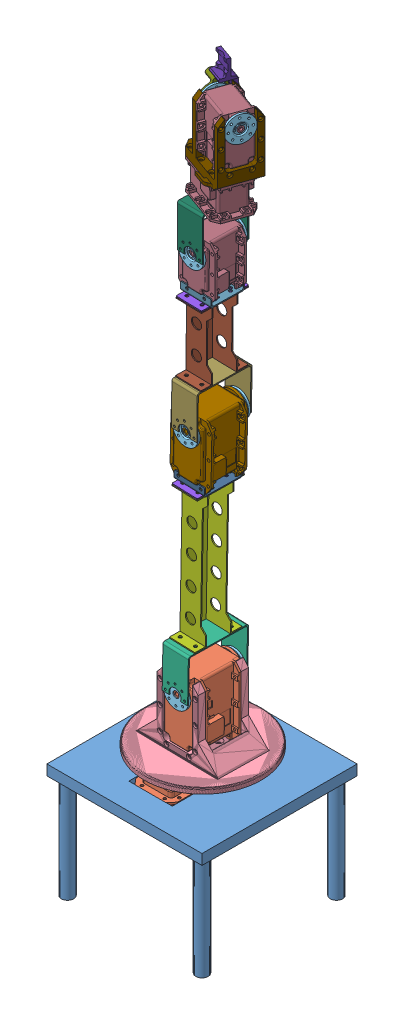
SolidWorks assembly assembly_crust_crawler, configuration Default. Lengths in mm.
Overall size (269.14 706.92 175.09).
38 component instances, 18 part files, 11 mates.
Components (placement in the parent):
- Assem1-1: Assem1 [Default] at (104.615 46.97 110.75) size (150 123.8 150)
  - Base-1: Base [Default] at (7.7733 111.5492 148.5502) size (150 110 150)
  - MX-106T-1: MX-106T [Default] at (7.7733 104.5492 147.8002) x (1 0 0) z (0 1 0) size (40.2 65.92 55.3)
  - Assem2^Assem1-1: Assem2^Assem1 [Default] at origin (virtual)
- Assem2-1: Assem2 [Default] at (121.2155 149.8024 367.5968) x (-0.955636 0 -0.294549) z (0.294549 0 -0.955636) size (140.05 72.32 140.05)
  - Base-disc-1: Base-disc [Default] at (40.5552 32.0167 101.6089) size (110 1 110)
  - NewBase.step-1: NewBase.step [Default] at (40.6801 33.4506 101.0855) x (0.960222 0 -0.279236) z (0 1 0) size (112.99 113 71)
  - MX-106T-1: MX-106T [Default] at (40.5074 89.0167 101.5981) x (0.960332 0 -0.27886) z (0.27886 0 0.960332) size (40.2 65.92 55.3)
- Assem3-1: Assem3 [Default] at (130.0492 256.093 286.4579) x (0.016376 0 -0.999866) z (-0.693879 0.720002 -0.011365) size (57.3 192.03 192.03)
  - Servo-Disc-1: Servo-Disc [Default] at (2.0912 25 0.1048) size (2 25 25)
  - Servo-Disc-2: Servo-Disc [Default] at (55.3912 25 0.1048) size (2 25 25)
  - Servo-disc-link_MX-106T-1: Servo-disc-link_MX-106T [Default] at (23.5912 -10.7089 18.136) x (1 0 0) z (0 -0.707107 0.707107) size (57.3 25 41)
  - Link-1-2: Link-1 [Default] at (29.7412 -39.3467 82.1292) x (-1 0 0) z (0 -0.707107 0.707107) size (45 25 130)
  - Link-plate-1: Link-plate [Default] at (29.7412 -94.1475 119.2523) x (1 0 0) z (0 -0.707107 0.707107) size (45 25 1)
  - MX-64T-1: MX-64T [Default] at (29.7412 -130.4221 155.5269) x (0 0.707107 0.707107) z (1 0 0) size (40.2 62.1 50)
  - Servo-link-link_MX-64T-1: Servo-link-link_MX-64T [Default] at (34.2412 -84.6016 130.9195) x (1 0 0) z (0 0.707107 -0.707107) size (36 30 8)
- Assem4-1: Assem4 [Default] at (-247.2098 484.9674 396.4744) x (-0.54317 0.771927 -0.330296) z (0.201622 -0.261959 -0.943783) size (161.15 123.42 91.84)
  - Link-plate-1: Link-plate [Default] at (-89.9377 341.0305 187.0442) x (0.321357 0 0.946958) z (0.767934 0.585117 -0.260604) size (45 25 1)
  - Link-2-1: Link-2 [Default] at (-108.7375 311.2922 193.4241) x (-0.321357 0 -0.946958) z (0.767934 0.585117 -0.260604) size (45 25 67)
  - Servo-Disc-1: Servo-Disc [Default] at (-178.346 279.3006 192.7579) x (-0.321357 0 -0.946958) z (0.934807 -0.159687 -0.317233) size (2 25 25)
  - Servo-disc-link_MX-64T-1: Servo-disc-link_MX-64T [Default] at (-133.7226 291.3982 205.5989) x (-0.321357 0 -0.946958) z (0.767934 0.585117 -0.260604) size (52 25 41)
  - Servo-Disc-2: Servo-Disc [Default] at (-163.5636 279.3006 236.318) x (0.321357 0 0.946958) z (0.288069 0.952607 -0.097758) size (2 25 25)
  - MX-28T-2: MX-28T [Default] at (-57.8381 365.4884 176.151) x (0.554082 -0.810949 -0.188031) z (0.321357 0 0.946958) size (35.6 50.71 41.85)
  - ConnectorThing.step-1: ConnectorThing.step [Default] at (-169.9614 278.7011 214.2008) x (0.767934 0.585117 -0.260604) z (0.321357 0 0.946958) size (8 30 32)
- Assem5-1: Assem5 [Default] at (242.9965 249.3023 120.2555) x (0.936637 0.049526 0.346782) z (-0.346377 -0.016805 0.937945) size (40.29 54.45 50.34)
  - Servo-Disc-1: Servo-Disc [Default] at (-51.4186 402.8975 162.088) x (-0.049717 -0.998621 0.016872) z (0.75968 -0.048777 -0.648465) size (2 25 25)
  - Servo-disc-link_MX-28T-1: Servo-disc-link_MX-28T [Default] at (-63.1296 401.0569 166.8098) x (0.331397 -0.000558 0.943491) z (0.049717 0.998621 -0.016872) size (43.85 25 41)
  - Servo-Disc-2: Servo-Disc [Default] at (-59.7039 362.4639 144.9157) x (-0.331397 0.000558 -0.943491) z (0.942181 -0.052499 -0.330967) size (2 25 25)
  - Servo-Disc-3: Servo-Disc [Default] at (-47.1605 362.4428 180.6269) x (0.331397 -0.000558 0.943491) z (0.942181 -0.052499 -0.330967) size (2 25 25)
- Assem6-1: Assem6 [Default] at (304.884 229.3011 269.5556) x (0.396254 0.049634 0.916798) z (-0.917472 -0.016687 0.397449) size (72.73 122.97 69.71)
  - Gripper2.step-1: Gripper2.step [Default] at (51.5353 645.8334 59.8001) x (-0.722497 0.121196 -0.680669) z (0.120066 0.991551 0.049105) size (28 15.5 49.84)
  - Gripper1.step-1: Gripper1.step [Default] at (27.7351 350.7975 53.5613) x (0.730716 -0.024853 0.682229) z (-0.049717 -0.998621 0.016872) size (17.31 15.51 73.9)
  - MX-28T-1: MX-28T [Default] at (-46.7712 504.3543 138.9568) x (0.730716 -0.024853 0.682229) z (-0.680869 0.046247 0.730944) size (35.6 50.71 41.85)
  - Servo-Disc-1: Servo-Disc [Default] at (-35.0263 503.5565 126.3481) x (0.680869 -0.046247 -0.730944) z (0.437057 -0.775176 0.456161) size (2 25 25)
  - Servo-Disc-2: Servo-Disc [Default] at (-60.7971 505.307 154.0143) x (-0.680869 0.046247 0.730944) z (0.732405 0.043319 0.679489) size (2 25 25)
  - Holder-thing.step-1: Holder-thing.step [Default] at (27.3796 352.5751 54.0069) x (0.730716 -0.024853 0.682229) z (-0.049717 -0.998621 0.016872) size (39.6 57 61.2)
  - MX-28T-2: MX-28T [Default] at (-66.9848 441.399 158.3136) x (0.730716 -0.024853 0.682229) z (-0.049717 -0.998621 0.016872) size (35.6 50.71 41.85)
  - Servo-Disc-3: Servo-Disc [Default] at (-66.1272 458.6252 158.0226) x (0.049717 0.998621 -0.016872) z (0.847678 -0.033257 0.529468) size (2 25 25)
Mates (geometry in assembly coordinates):
- Concentric2: concentric aligned: circle of Assem1-1/MX-106T-1; circle of Assem2-1/Base-disc-1
- Coincident3: coincident anti-aligned: plane of Assem1-1/MX-106T-1 through (115.2522 182.3192 255.6862) normal (0 1 0); plane of Assem2-1/NewBase.step-1 through (112.3883 182.3192 258.5501) normal (0 -1 0)
- Concentric3: concentric aligned: circle of Assem2-1/MX-106T-1; circle of Assem3-1/Servo-Disc-2
- Coincident7: coincident anti-aligned: plane of Assem2-1/MX-106T-1 through (107.6867 244.0192 230.6931) normal (0.016376 0 -0.999866); plane of Assem3-1/Servo-Disc-2 through (112.886 238.8192 230.7782) normal (-0.016376 0 0.999866)
- Concentric5: concentric aligned: circle of Assem3-1/MX-64T-1; circle of Assem4-1/Servo-Disc-2
- Concentric6: concentric aligned: circle of Assem3-1/MX-64T-1; circle of Assem4-1/Servo-Disc-2
- Coincident9: coincident anti-aligned: plane of Assem3-1/MX-64T-1 through (111.8146 463.8769 231.1107) normal (0.016376 0 -0.999866); plane of Assem4-1/Servo-Disc-2 through (116.9254 458.5819 231.1944) normal (-0.016376 0 0.999866)
- Concentric7: concentric aligned: circle of Assem4-1/MX-28T-2; circle of Assem5-1/Servo-Disc-2
- Distance2: distance = 1.5 mm anti-aligned: plane of Assem4-1/MX-28T-2 through (129.3141 572.9346 236.648) normal (0.016376 0 -0.999866); plane of Assem5-1/Servo-Disc-2 through (117.9305 605.8781 234.9614) normal (-0.016376 0 0.999866)
- Concentric8: concentric aligned: circle of Assem5-1/Servo-Disc-1; circle of Assem6-1/MX-28T-2
- Coincident11: coincident anti-aligned: plane of Assem5-1/Servo-Disc-1 through (117.6288 646.3781 253.884) normal (0.000203 1 0.000003); plane of Assem6-1/MX-28T-2 through (152.4921 646.371 253.9359) normal (-0.000203 -1 -0.000003)
